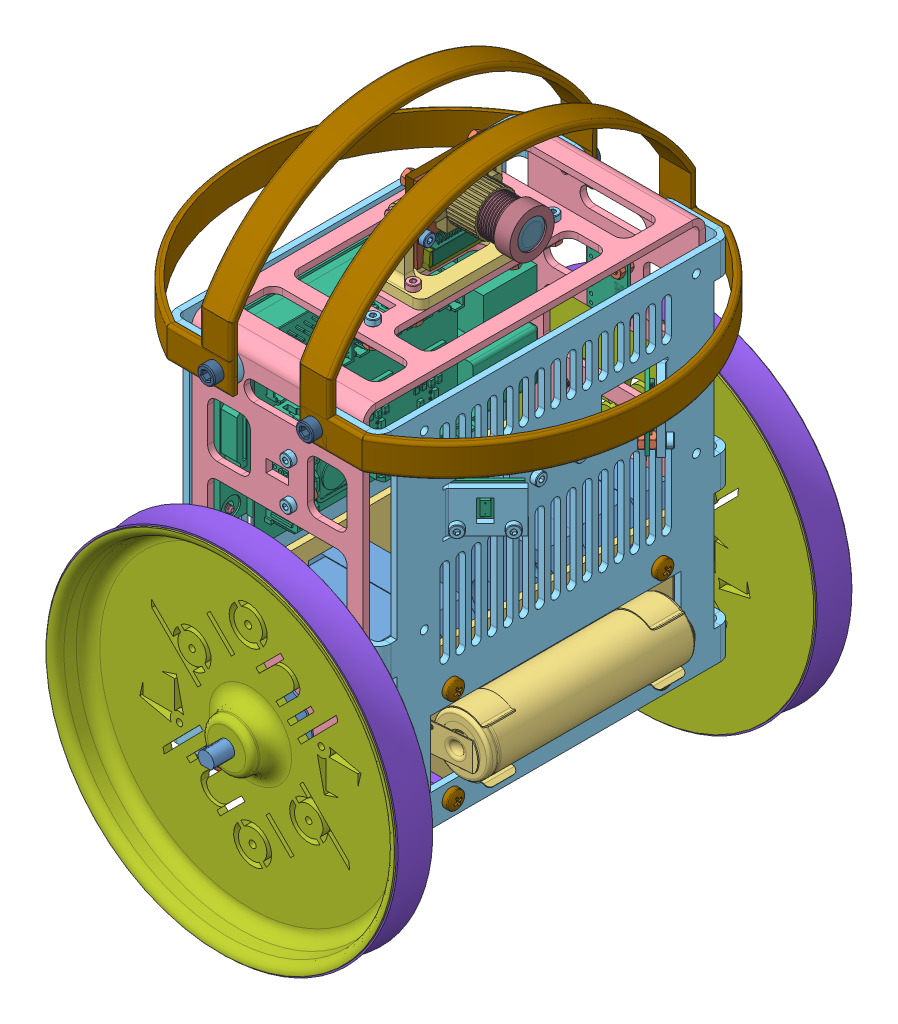
SolidWorks assembly irys4, configuration Domyślna. Lengths in mm.
Overall size (174.89 215.39 153).
175 component instances, 30 part files, 180 mates.
Components (placement in the parent):
- steppermotor-1: steppermotor [Default] at (-42.2578 -7.1789 72.25) size (42.3 42.3 64.5)
- bottomframe_rys3-1: bottomframe_rys3 [Domyślna] at (-43.1924 -30.5373 18.7182) x (0 0 -1) z (0 -1 0) size (108 54 24.86)
- steppermotor-2: steppermotor [Default] at (-42.2578 -7.1789 -31.75) x (-1 0 0) z (0 0 -1) size (42.3 42.3 64.5)
- battery_module-1: battery_module [Domyślna] at (-62.2578 -30.5373 65.25) x (0 0 -1) z (0 -1 0) size (90 40 22.7)
- topframe-1: topframe [Domyślna] at (-42.6117 88.6087 10.8622) x (0 0 -1) z (0 1 0) size (108 54 97.29)
- front-1: front [Domyślna] at (-98.6996 69.3173 29.4239) x (0.707107 0 0.707107) z (0 -1 0) size (94.01 94.01 115)
- rys_PCB_rpi_simple-1: rys_PCB_rpi_simple [Domyślna] at (-55.33 110.1932 110.0692) x (0 -1 0) z (1 0 0) size (61.22 87.74 23.25)
- front-2: front [Domyślna] at (14.1841 69.3173 11.0761) x (-0.707107 0 -0.707107) z (0 -1 0) size (94.01 94.01 115)
- wheel wide wide-1: wheel wide wide [bionik x2] at (-42.2578 18.6 82.75) x (0 0 1) z (-1 0 0) size (12 110 110)
- wheel wide wide-2: wheel wide wide [bionik x2] at (-42.3556 18.5998 -42.5179) x (0 0 -1) z (0.999993 0.003797 0) size (12 110 110)
- tire wide-1: tire wide [Domyślna] at (-42.2578 -7.1789 -35.7326) x (0 0 -1) z (0.906427 0.422363 0) size (11 111 111)
- tire wide-2: tire wide [Domyślna] at (-42.2578 -7.1789 96.4849) x (0 0 -1) z (0.998984 -0.045072 0) size (11 111 111)
- bumper-2: bumper [Domyślna] at (-72.7578 82.3211 20.318) x (0 0 1) z (0 -1 0) size (116 57.13 10)
- bumper-3: bumper [Domyślna] at (-11.7578 82.3211 20.25) x (0 0 1) z (0 1 0) size (116 57.13 10)
- imu-1: imu [Domyślna] at (-53.5985 -9.4799 25.3181) x (-0.019519 0 -0.999809) z (0 -1 0) size (10.16 22.86 2.23)
- camera_mounted-1: camera_mounted [Domyślna] at (-47.1687 108.7904 16.7906) x (0 0 -1) z (0.999935 0.011413 0) size (36.3 30.27 33.11)
  - Camera Module Assem-1: Camera Module Assem [Default] at (-12.4357 -13.5775 -13.0743) size (25 24 24.98)
    - PCB 1-1: PCB 1 [Default] at (8.9736 12.851 19.5114) size (25 24 2.1)
    - Camera Block-1: Camera Block [Default] at (8.9736 15.851 20.5114) size (22 13.5 12.5)
    - Camera end-1: Camera end [Default] at (8.9736 15.851 27.3922) x (0.999924 0.012337 0) z (0 0 1) size (14 14 17.26)
    - Lenz-1: Lenz [Default] at (8.9736 15.851 43.8922) size (9 9 0.5)
    - 15 Pin Ribbon Block Assem-1: 15 Pin Ribbon Block Assem [Default] at (0.7567 20.5462 10.9417) x (1 0 0) z (0 -1 0) size (22 2.5 7)
      - 15 Pin Ribbon Block-1: 15 Pin Ribbon Block [Default] at (8.217 10.8197 14.6952) size (20 2.5 6)
      - Ribbon Clamp-1: Ribbon Clamp [Default] at (8.217 10.8197 14.6952) size (22 2.5 5)
    - 0603 Resistor-1: 0603 Resistor [Default] at (2.3268 23.572 20.4882) size (1.75 0.89 0.66)
    - 0603 Resistor-2: 0603 Resistor [Default] at (4.5768 23.572 20.4882) size (1.75 0.89 0.66)
    - 0603 Resistor-3: 0603 Resistor [Default] at (15.6203 23.5707 20.4857) size (1.75 0.89 0.66)
    - 0603 Resistor-4: 0603 Resistor [Default] at (13.3703 23.5707 20.4857) size (1.75 0.89 0.66)
  - mount-1: mount [Domyślna] at (-15.8432 -12.9016 1.4371) size (25 24 5)
  - M2 x 0.4mm Thread 5mm LONG SOCKET HEAD CAP SCREW-1: M2 x 0.4mm Thread 5mm LONG SOCKET HEAD CAP SCREW [Domyślna] at (7.0379 9.2735 2.5371) x (-0.356462 0.93431 0) z (0 0 -1) size (3.8 3.8 7.09)
  - M2 x 0.4mm Thread 5mm LONG SOCKET HEAD CAP SCREW-2: M2 x 0.4mm Thread 5mm LONG SOCKET HEAD CAP SCREW [Domyślna] at (7.0379 -4.7265 2.5371) x (-0.994039 0.109029 0) z (0 0 -1) size (3.8 3.8 7.09)
  - M2 x 0.4mm Thread 5mm LONG SOCKET HEAD CAP SCREW-3: M2 x 0.4mm Thread 5mm LONG SOCKET HEAD CAP SCREW [Domyślna] at (-13.9621 9.2735 2.5371) x (-0.583934 -0.811801 0) z (0 0 -1) size (3.8 3.8 7.09)
  - M2 x 0.4mm Thread 5mm LONG SOCKET HEAD CAP SCREW-4: M2 x 0.4mm Thread 5mm LONG SOCKET HEAD CAP SCREW [Domyślna] at (-13.9621 -4.7265 2.5371) x (-0.923728 -0.383049 0) z (0 0 -1) size (3.8 3.8 7.09)
  - m2_x_0_4mm_thread_hex_nut-1: m2_x_0_4mm_thread_hex_nut [Domyślna] at (7.0379 9.2735 3.1371) size (4 4.62 1.6)
  - m2_x_0_4mm_thread_hex_nut-2: m2_x_0_4mm_thread_hex_nut [Domyślna] at (7.0379 -4.7265 3.1371) size (4 4.62 1.6)
  - m2_x_0_4mm_thread_hex_nut-3: m2_x_0_4mm_thread_hex_nut [Domyślna] at (-13.9621 -4.7265 3.1371) size (4 4.62 1.6)
  - m2_x_0_4mm_thread_hex_nut-4: m2_x_0_4mm_thread_hex_nut [Domyślna] at (-13.9621 9.2735 3.1371) size (4 4.62 1.6)
  - mount1-1: mount1 [Domyślna] at (7.7442 -6.03 1.3422) x (1 0 0) z (0 -0.011413 0.999935) size (36.3 23 16)
  - M2 x 0.4mm Thread 10mm LONG SOCKET HEAD CAP SCREW-1: M2 x 0.4mm Thread 10mm LONG SOCKET HEAD CAP SCREW [Domyślna] at (1.9591 2.2735 3.9371) x (0 0.966896 -0.255169) z (-1 0 0) size (3.8 3.8 12.09)
  - M2 x 0.4mm Thread 10mm LONG SOCKET HEAD CAP SCREW-2: M2 x 0.4mm Thread 10mm LONG SOCKET HEAD CAP SCREW [Domyślna] at (-8.8833 2.2735 3.9371) x (0 0 -1) z (1 0 0) size (3.8 3.8 12.09)
- bumper-4: bumper [Domyślna] at (-57.7497 97.3211 20.25) x (0 0 1) z (-1 0.000537 0) size (116 57.13 10)
- bumper-5: bumper [Domyślna] at (-26.7108 97.321 20.25) x (0 0 1) z (-0.999995 0.003129 0) size (116 57.13 10)
- m2_x_0_4mm_thread_6mm_long_sock-1: m2_x_0_4mm_thread_6mm_long_sock [Domyślna] at (-11.1317 52.3211 48.7547) x (-0.511229 -0.690862 0.511229) z (-0.707107 0 -0.707107) size (3.8 3.8 8)
- m2_x_0_4mm_thread_6mm_long_sock-2: m2_x_0_4mm_thread_6mm_long_sock [Domyślna] at (-2.1514 52.3211 39.7744) x (-0.511229 -0.690862 0.511229) z (-0.707107 0 -0.707107) size (3.8 3.8 8)
- M2 x 0.4mm Thread 10mm LONG SOCKET HEAD CAP SCREW-1: M2 x 0.4mm Thread 10mm LONG SOCKET HEAD CAP SCREW [Domyślna] at (-66.0454 33.0917 64.6663) x (0 -0.924225 -0.381849) z (1 0 0) size (3.8 3.8 12.09)
- M2 x 0.4mm Thread 10mm LONG SOCKET HEAD CAP SCREW-2: M2 x 0.4mm Thread 10mm LONG SOCKET HEAD CAP SCREW [Domyślna] at (-66.0454 82.1645 64.6663) x (0 -0.924225 -0.381849) z (1 0 0) size (3.8 3.8 12.09)
- ToF_nut-1: ToF_nut [Domyślna] at (-17.0376 55.6897 33.0308) x (0 -1 0) z (0.707107 0 0.707107) size (12.89 18.5 4.22)
  - vl53l1x-1: vl53l1x [Domyślna] at (-6.7913 -9.4823 16.6745) size (12.7 17.78 2.22)
  - m2_x_0_4mm_thread_hex_nut-1: m2_x_0_4mm_thread_hex_nut [Domyślna] at (3.3687 5.7577 15.8745) size (4 4.62 1.6)
  - m2_x_0_4mm_thread_hex_nut-2: m2_x_0_4mm_thread_hex_nut [Domyślna] at (3.3687 -6.9423 15.8745) x (-0.923728 -0.383049 0) z (0 0 -1) size (4 4.62 1.6)
  - m2_x_0_4mm_thread_hex_nut-3: m2_x_0_4mm_thread_hex_nut [Domyślna] at (3.3687 5.7577 18.4945) x (-0.923728 -0.383049 0) z (0 0 -1) size (4 4.62 1.6)
  - m2_x_0_4mm_thread_hex_nut-4: m2_x_0_4mm_thread_hex_nut [Domyślna] at (3.3687 -6.9423 18.4945) x (-0.923728 -0.383049 0) z (0 0 -1) size (4 4.62 1.6)
- ToF_nut-2: ToF_nut [Domyślna] at (-17.6432 55.6897 6.5354) x (0 -1 0) z (0.707107 0 -0.707107) size (12.89 18.5 4.22)
  - vl53l1x-1: vl53l1x [Domyślna] at (-6.7913 -9.4823 16.6745) size (12.7 17.78 2.22)
  - m2_x_0_4mm_thread_hex_nut-1: m2_x_0_4mm_thread_hex_nut [Domyślna] at (3.3687 5.7577 15.8745) size (4 4.62 1.6)
  - m2_x_0_4mm_thread_hex_nut-2: m2_x_0_4mm_thread_hex_nut [Domyślna] at (3.3687 -6.9423 15.8745) x (-0.923728 -0.383049 0) z (0 0 -1) size (4 4.62 1.6)
  - m2_x_0_4mm_thread_hex_nut-3: m2_x_0_4mm_thread_hex_nut [Domyślna] at (3.3687 5.7577 18.4945) x (-0.923728 -0.383049 0) z (0 0 -1) size (4 4.62 1.6)
  - m2_x_0_4mm_thread_hex_nut-4: m2_x_0_4mm_thread_hex_nut [Domyślna] at (3.3687 -6.9423 18.4945) x (-0.923728 -0.383049 0) z (0 0 -1) size (4 4.62 1.6)
- ToF_nut-3: ToF_nut [Domyślna] at (-29.7647 55.6897 19.6577) x (0 -1 0) z (1 0 0) size (12.89 18.5 4.22)
  - vl53l1x-1: vl53l1x [Domyślna] at (-6.7913 -9.4823 16.6745) size (12.7 17.78 2.22)
  - m2_x_0_4mm_thread_hex_nut-1: m2_x_0_4mm_thread_hex_nut [Domyślna] at (3.3687 5.7577 15.8745) size (4 4.62 1.6)
  - m2_x_0_4mm_thread_hex_nut-2: m2_x_0_4mm_thread_hex_nut [Domyślna] at (3.3687 -6.9423 15.8745) x (-0.923728 -0.383049 0) z (0 0 -1) size (4 4.62 1.6)
  - m2_x_0_4mm_thread_hex_nut-3: m2_x_0_4mm_thread_hex_nut [Domyślna] at (3.3687 5.7577 18.4945) x (-0.923728 -0.383049 0) z (0 0 -1) size (4 4.62 1.6)
  - m2_x_0_4mm_thread_hex_nut-4: m2_x_0_4mm_thread_hex_nut [Domyślna] at (3.3687 -6.9423 18.4945) x (-0.923728 -0.383049 0) z (0 0 -1) size (4 4.62 1.6)
- m2_x_0_4mm_thread_6mm_long_sock-3: m2_x_0_4mm_thread_6mm_long_sock [Domyślna] at (-14.4701 52.3211 13.9) x (0 0.924225 0.381849) z (-1 0 0) size (3.8 3.8 8)
- m2_x_0_4mm_thread_6mm_long_sock-4: m2_x_0_4mm_thread_6mm_long_sock [Domyślna] at (-10.8996 52.3211 -8.3508) x (0.65106 0.390182 0.65106) z (-0.707107 0 0.707107) size (3.8 3.8 8)
- m2_x_0_4mm_thread_6mm_long_sock-5: m2_x_0_4mm_thread_6mm_long_sock [Domyślna] at (-14.4701 52.3211 26.6) x (0 0.924225 0.381849) z (-1 0 0) size (3.8 3.8 8)
- m2_x_0_4mm_thread_6mm_long_sock-6: m2_x_0_4mm_thread_6mm_long_sock [Domyślna] at (-1.9194 52.3211 0.6295) x (0.693391 -0.196001 0.693391) z (-0.707107 0 0.707107) size (3.8 3.8 8)
- ToF_nut-4: ToF_nut [Domyślna] at (-41.1264 69.3142 -2.3423) x (1 0 0) z (0 1 0) size (12.89 18.5 4.22)
  - vl53l1x-1: vl53l1x [Domyślna] at (-6.7913 -9.4823 16.6745) size (12.7 17.78 2.22)
  - m2_x_0_4mm_thread_hex_nut-1: m2_x_0_4mm_thread_hex_nut [Domyślna] at (3.3687 5.7577 15.8745) size (4 4.62 1.6)
  - m2_x_0_4mm_thread_hex_nut-2: m2_x_0_4mm_thread_hex_nut [Domyślna] at (3.3687 -6.9423 15.8745) x (-0.923728 -0.383049 0) z (0 0 -1) size (4 4.62 1.6)
  - m2_x_0_4mm_thread_hex_nut-3: m2_x_0_4mm_thread_hex_nut [Domyślna] at (3.3687 5.7577 18.4945) x (-0.923728 -0.383049 0) z (0 0 -1) size (4 4.62 1.6)
  - m2_x_0_4mm_thread_hex_nut-4: m2_x_0_4mm_thread_hex_nut [Domyślna] at (3.3687 -6.9423 18.4945) x (-0.923728 -0.383049 0) z (0 0 -1) size (4 4.62 1.6)
- ToF_nut-5: ToF_nut [Domyślna] at (-41.1264 69.3142 41.6577) x (1 0 0) z (0 1 0) size (12.89 18.5 4.22)
  - vl53l1x-1: vl53l1x [Domyślna] at (-6.7913 -9.4823 16.6745) size (12.7 17.78 2.22)
  - m2_x_0_4mm_thread_hex_nut-1: m2_x_0_4mm_thread_hex_nut [Domyślna] at (3.3687 5.7577 15.8745) size (4 4.62 1.6)
  - m2_x_0_4mm_thread_hex_nut-2: m2_x_0_4mm_thread_hex_nut [Domyślna] at (3.3687 -6.9423 15.8745) x (-0.923728 -0.383049 0) z (0 0 -1) size (4 4.62 1.6)
  - m2_x_0_4mm_thread_hex_nut-3: m2_x_0_4mm_thread_hex_nut [Domyślna] at (3.3687 5.7577 18.4945) x (-0.923728 -0.383049 0) z (0 0 -1) size (4 4.62 1.6)
  - m2_x_0_4mm_thread_hex_nut-4: m2_x_0_4mm_thread_hex_nut [Domyślna] at (3.3687 -6.9423 18.4945) x (-0.923728 -0.383049 0) z (0 0 -1) size (4 4.62 1.6)
- M2 x 0.4mm Thread 10mm LONG SOCKET HEAD CAP SCREW-3: M2 x 0.4mm Thread 10mm LONG SOCKET HEAD CAP SCREW [Domyślna] at (-37.7578 83.6087 4.6) x (0.952226 0 0.305395) z (0 -1 0) size (3.8 3.8 12.09)
- M2 x 0.4mm Thread 10mm LONG SOCKET HEAD CAP SCREW-4: M2 x 0.4mm Thread 10mm LONG SOCKET HEAD CAP SCREW [Domyślna] at (-37.7578 83.6087 35.9) x (0.999568 0 -0.029375) z (0 -1 0) size (3.8 3.8 12.09)
- m2_x_0_4mm_thread_6mm_long_sock-7: m2_x_0_4mm_thread_6mm_long_sock [Domyślna] at (-37.7578 84.6087 48.6) x (-0.868702 0 -0.495335) z (0 -1 0) size (3.8 3.8 8)
- m2_x_0_4mm_thread_6mm_long_sock-8: m2_x_0_4mm_thread_6mm_long_sock [Domyślna] at (-37.7578 84.6087 -8.1) x (-0.837169 0 -0.546944) z (0 -1 0) size (3.8 3.8 8)
- ToF_nut-6: ToF_nut [Domyślna] at (-41.1264 60.9134 52.9555) size (12.89 18.5 4.22)
  - vl53l1x-1: vl53l1x [Domyślna] at (-6.7913 -9.4823 16.6745) size (12.7 17.78 2.22)
  - m2_x_0_4mm_thread_hex_nut-1: m2_x_0_4mm_thread_hex_nut [Domyślna] at (3.3687 5.7577 15.8745) size (4 4.62 1.6)
  - m2_x_0_4mm_thread_hex_nut-2: m2_x_0_4mm_thread_hex_nut [Domyślna] at (3.3687 -6.9423 15.8745) x (-0.923728 -0.383049 0) z (0 0 -1) size (4 4.62 1.6)
  - m2_x_0_4mm_thread_hex_nut-3: m2_x_0_4mm_thread_hex_nut [Domyślna] at (3.3687 5.7577 18.4945) x (-0.923728 -0.383049 0) z (0 0 -1) size (4 4.62 1.6)
  - m2_x_0_4mm_thread_hex_nut-4: m2_x_0_4mm_thread_hex_nut [Domyślna] at (3.3687 -6.9423 18.4945) x (-0.923728 -0.383049 0) z (0 0 -1) size (4 4.62 1.6)
- ToF_nut-7: ToF_nut [Domyślna] at (-41.1264 59.7288 -12.4555) x (1 0 0) z (0 0 -1) size (12.89 18.5 4.22)
  - vl53l1x-1: vl53l1x [Domyślna] at (-6.7913 -9.4823 16.6745) size (12.7 17.78 2.22)
  - m2_x_0_4mm_thread_hex_nut-1: m2_x_0_4mm_thread_hex_nut [Domyślna] at (3.3687 5.7577 15.8745) size (4 4.62 1.6)
  - m2_x_0_4mm_thread_hex_nut-2: m2_x_0_4mm_thread_hex_nut [Domyślna] at (3.3687 -6.9423 15.8745) x (-0.923728 -0.383049 0) z (0 0 -1) size (4 4.62 1.6)
  - m2_x_0_4mm_thread_hex_nut-3: m2_x_0_4mm_thread_hex_nut [Domyślna] at (3.3687 5.7577 18.4945) x (-0.923728 -0.383049 0) z (0 0 -1) size (4 4.62 1.6)
  - m2_x_0_4mm_thread_hex_nut-4: m2_x_0_4mm_thread_hex_nut [Domyślna] at (3.3687 -6.9423 18.4945) x (-0.923728 -0.383049 0) z (0 0 -1) size (4 4.62 1.6)
- ToF_nut-8: ToF_nut [Domyślna] at (-67.478 55.6897 7.4692) x (0 -1 0) z (-0.707107 0 -0.707107) size (12.89 18.5 4.22)
  - vl53l1x-1: vl53l1x [Domyślna] at (-6.7913 -9.4823 16.6745) size (12.7 17.78 2.22)
  - m2_x_0_4mm_thread_hex_nut-1: m2_x_0_4mm_thread_hex_nut [Domyślna] at (3.3687 5.7577 15.8745) size (4 4.62 1.6)
  - m2_x_0_4mm_thread_hex_nut-2: m2_x_0_4mm_thread_hex_nut [Domyślna] at (3.3687 -6.9423 15.8745) x (-0.923728 -0.383049 0) z (0 0 -1) size (4 4.62 1.6)
  - m2_x_0_4mm_thread_hex_nut-3: m2_x_0_4mm_thread_hex_nut [Domyślna] at (3.3687 5.7577 18.4945) x (-0.923728 -0.383049 0) z (0 0 -1) size (4 4.62 1.6)
  - m2_x_0_4mm_thread_hex_nut-4: m2_x_0_4mm_thread_hex_nut [Domyślna] at (3.3687 -6.9423 18.4945) x (-0.923728 -0.383049 0) z (0 0 -1) size (4 4.62 1.6)
- ToF_nut-9: ToF_nut [Domyślna] at (-54.7508 55.6897 20.8423) x (0 -1 0) z (-1 0 0) size (12.89 18.5 4.22)
  - vl53l1x-1: vl53l1x [Domyślna] at (-6.7913 -9.4823 16.6745) size (12.7 17.78 2.22)
  - m2_x_0_4mm_thread_hex_nut-1: m2_x_0_4mm_thread_hex_nut [Domyślna] at (3.3687 5.7577 15.8745) size (4 4.62 1.6)
  - m2_x_0_4mm_thread_hex_nut-2: m2_x_0_4mm_thread_hex_nut [Domyślna] at (3.3687 -6.9423 15.8745) x (-0.923728 -0.383049 0) z (0 0 -1) size (4 4.62 1.6)
  - m2_x_0_4mm_thread_hex_nut-3: m2_x_0_4mm_thread_hex_nut [Domyślna] at (3.3687 5.7577 18.4945) x (-0.923728 -0.383049 0) z (0 0 -1) size (4 4.62 1.6)
  - m2_x_0_4mm_thread_hex_nut-4: m2_x_0_4mm_thread_hex_nut [Domyślna] at (3.3687 -6.9423 18.4945) x (-0.923728 -0.383049 0) z (0 0 -1) size (4 4.62 1.6)
- ToF_nut-10: ToF_nut [Domyślna] at (-66.8723 55.6897 33.9646) x (0 -1 0) z (-0.707107 0 0.707107) size (12.89 18.5 4.22)
  - vl53l1x-1: vl53l1x [Domyślna] at (-6.7913 -9.4823 16.6745) size (12.7 17.78 2.22)
  - m2_x_0_4mm_thread_hex_nut-1: m2_x_0_4mm_thread_hex_nut [Domyślna] at (3.3687 5.7577 15.8745) size (4 4.62 1.6)
  - m2_x_0_4mm_thread_hex_nut-2: m2_x_0_4mm_thread_hex_nut [Domyślna] at (3.3687 -6.9423 15.8745) x (-0.923728 -0.383049 0) z (0 0 -1) size (4 4.62 1.6)
  - m2_x_0_4mm_thread_hex_nut-3: m2_x_0_4mm_thread_hex_nut [Domyślna] at (3.3687 5.7577 18.4945) x (-0.923728 -0.383049 0) z (0 0 -1) size (4 4.62 1.6)
  - m2_x_0_4mm_thread_hex_nut-4: m2_x_0_4mm_thread_hex_nut [Domyślna] at (3.3687 -6.9423 18.4945) x (-0.923728 -0.383049 0) z (0 0 -1) size (4 4.62 1.6)
- m2_x_0_4mm_thread_6mm_long_sock-9: m2_x_0_4mm_thread_6mm_long_sock [Domyślna] at (-73.3839 52.3211 -8.2547) x (0.707107 0 -0.707107) z (0.707107 0 0.707107) size (3.8 3.8 8)
- m2_x_0_4mm_thread_6mm_long_sock-10: m2_x_0_4mm_thread_6mm_long_sock [Domyślna] at (-82.3641 52.3211 0.7256) x (0.403735 0.820972 -0.403735) z (0.707107 0 0.707107) size (3.8 3.8 8)
- m2_x_0_4mm_thread_6mm_long_sock-11: m2_x_0_4mm_thread_6mm_long_sock [Domyślna] at (-70.0454 52.3211 13.9) x (0 -0.924225 -0.381849) z (1 0 0) size (3.8 3.8 8)
- m2_x_0_4mm_thread_6mm_long_sock-12: m2_x_0_4mm_thread_6mm_long_sock [Domyślna] at (-70.0454 52.3211 26.6) x (0 -0.924225 -0.381849) z (1 0 0) size (3.8 3.8 8)
- m2_x_0_4mm_thread_6mm_long_sock-13: m2_x_0_4mm_thread_6mm_long_sock [Domyślna] at (-82.5962 52.3211 39.8705) x (0.184692 -0.965286 0.184692) z (0.707107 0 -0.707107) size (3.8 3.8 8)
- m2_x_0_4mm_thread_6mm_long_sock-14: m2_x_0_4mm_thread_6mm_long_sock [Domyślna] at (-73.6159 52.3211 48.8508) x (-0.648462 -0.398739 -0.648462) z (0.707107 0 -0.707107) size (3.8 3.8 8)
- m2_x_0_4mm_thread_6mm_long_sock-15: m2_x_0_4mm_thread_6mm_long_sock [Domyślna] at (-37.7578 66.6711 68.25) x (-0.262854 -0.964836 0) z (0 0 -1) size (3.8 3.8 8)
- m2_x_0_4mm_thread_6mm_long_sock-16: m2_x_0_4mm_thread_6mm_long_sock [Domyślna] at (-37.7578 53.9711 68.25) x (0.638921 -0.769272 0) z (0 0 -1) size (3.8 3.8 8)
- m2_x_0_4mm_thread_6mm_long_sock-17: m2_x_0_4mm_thread_6mm_long_sock [Domyślna] at (-37.7578 66.6711 -27.75) size (3.8 3.8 8)
- m2_x_0_4mm_thread_6mm_long_sock-18: m2_x_0_4mm_thread_6mm_long_sock [Domyślna] at (-37.7578 53.9711 -27.75) size (3.8 3.8 8)
- H-H_M3x12mm-1: H-H_M3x12mm [Predeterminado] at (-51.2078 -22.4959 17.65) x (0.837169 0 0.546944) z (0.546944 0 -0.837169) size (5.77 12 5)
- H-H_M3x6mm-1: H-H_M3x6mm [Predeterminado] at (-51.2078 -13.4959 17.65) x (0.837169 0 0.546944) z (0.546944 0 -0.837169) size (5.77 6 5)
- pan cross head_am-2: pan cross head_am [B18.6.7M - M3 x 0.5 x 6 Type I Cross Recessed PHMS --6N] at (-51.2078 -7.0799 17.65) x (0 -1 0) z (0 0 1) size (8.37 5.6 5.6)
- battery_module_H-2: battery_module_H [Domyślna] at (13.655 -6.0808 19.8906) x (0 0 1) z (-1 0 0) size (90 40 24.06)
  - battery_module-1: battery_module [Domyślna] at (-44.6406 -21.0981 81.7004) size (90 40 22.7)
  - H-H_M3x6mm-1: H-H_M3x6mm [Predeterminado] at (-32.6406 13.9019 84.7004) x (1 0 0) z (0 1 0) size (5.77 6 5)
  - H-H_M3x6mm-2: H-H_M3x6mm [Predeterminado] at (33.3594 13.9019 84.7004) x (1 0 0) z (0 1 0) size (5.77 6 5)
  - H-H_M3x6mm-3: H-H_M3x6mm [Predeterminado] at (-32.6406 -16.0981 84.7004) x (1 0 0) z (0 -1 0) size (5.77 6 5)
  - H-H_M3x6mm-4: H-H_M3x6mm [Predeterminado] at (33.3594 -16.0981 84.7004) x (1 0 0) z (0 1 0) size (5.77 6 5)
  - pan cross head_am-1: pan cross head_am [B18.6.7M - M3 x 0.5 x 6 Type I Cross Recessed PHMS --6N] at (-32.6406 -16.0981 77.2589) x (0 0 1) z (-1 0 0) size (8.37 5.6 5.6)
  - pan cross head_am-3: pan cross head_am [B18.6.7M - M3 x 0.5 x 6 Type I Cross Recessed PHMS --6N] at (-32.6406 13.9019 77.2589) x (0 0 1) z (-1 0 0) size (8.37 5.6 5.6)
  - pan cross head_am-4: pan cross head_am [B18.6.7M - M3 x 0.5 x 6 Type I Cross Recessed PHMS --6N] at (33.3594 13.9019 77.2589) x (0 0 1) z (-1 0 0) size (8.37 5.6 5.6)
  - pan cross head_am-5: pan cross head_am [B18.6.7M - M3 x 0.5 x 6 Type I Cross Recessed PHMS --6N] at (33.3594 -16.0981 77.2589) x (0 0 1) z (-1 0 0) size (8.37 5.6 5.6)
- pan cross head_am-3: pan cross head_am [B18.6.7M - M3 x 0.5 x 6 Type I Cross Recessed PHMS --6N] at (-78.4454 -22.1789 53.25) size (8.37 5.6 5.6)
- pan cross head_am-4: pan cross head_am [B18.6.7M - M3 x 0.5 x 6 Type I Cross Recessed PHMS --6N] at (-78.4454 7.8211 53.25) size (8.37 5.6 5.6)
- pan cross head_am-5: pan cross head_am [B18.6.7M - M3 x 0.5 x 6 Type I Cross Recessed PHMS --6N] at (-78.4454 7.8211 -12.75) size (8.37 5.6 5.6)
- pan cross head_am-6: pan cross head_am [B18.6.7M - M3 x 0.5 x 6 Type I Cross Recessed PHMS --6N] at (-78.4454 -22.1789 -12.75) size (8.37 5.6 5.6)
- pan cross head_am-7: pan cross head_am [B18.6.7M - M3 x 0.5 x 6 Type I Cross Recessed PHMS --6N] at (-57.2578 -34.9373 53.25) x (0 1 0) z (0 0 1) size (8.37 5.6 5.6)
- pan cross head_am-8: pan cross head_am [B18.6.7M - M3 x 0.5 x 6 Type I Cross Recessed PHMS --6N] at (-27.2578 -34.9373 53.25) x (0 1 0) z (0 0 1) size (8.37 5.6 5.6)
- pan cross head_am-9: pan cross head_am [B18.6.7M - M3 x 0.5 x 6 Type I Cross Recessed PHMS --6N] at (-57.2578 -34.9373 -12.75) x (0 1 0) z (0 0 1) size (8.37 5.6 5.6)
- pan cross head_am-10: pan cross head_am [B18.6.7M - M3 x 0.5 x 6 Type I Cross Recessed PHMS --6N] at (-27.2578 -34.9373 -12.75) x (0 1 0) z (0 0 1) size (8.37 5.6 5.6)
- battery_module_H-3: battery_module_H [Domyślna] at (-98.1705 -8.277 19.8906) x (0 0 1) z (1 0 0) size (90 40 24.06)
  - battery_module-1: battery_module [Domyślna] at (-44.6406 -21.0981 81.7004) size (90 40 22.7)
  - H-H_M3x6mm-1: H-H_M3x6mm [Predeterminado] at (-32.6406 13.9019 84.7004) x (1 0 0) z (0 1 0) size (5.77 6 5)
  - H-H_M3x6mm-2: H-H_M3x6mm [Predeterminado] at (33.3594 13.9019 84.7004) x (1 0 0) z (0 1 0) size (5.77 6 5)
  - H-H_M3x6mm-3: H-H_M3x6mm [Predeterminado] at (-32.6406 -16.0981 84.7004) x (1 0 0) z (0 -1 0) size (5.77 6 5)
  - H-H_M3x6mm-4: H-H_M3x6mm [Predeterminado] at (33.3594 -16.0981 84.7004) x (1 0 0) z (0 1 0) size (5.77 6 5)
  - pan cross head_am-1: pan cross head_am [B18.6.7M - M3 x 0.5 x 6 Type I Cross Recessed PHMS --6N] at (-32.6406 -16.0981 77.2589) x (0 0 1) z (-1 0 0) size (8.37 5.6 5.6)
  - pan cross head_am-3: pan cross head_am [B18.6.7M - M3 x 0.5 x 6 Type I Cross Recessed PHMS --6N] at (-32.6406 13.9019 77.2589) x (0 0 1) z (-1 0 0) size (8.37 5.6 5.6)
  - pan cross head_am-4: pan cross head_am [B18.6.7M - M3 x 0.5 x 6 Type I Cross Recessed PHMS --6N] at (33.3594 13.9019 77.2589) x (0 0 1) z (-1 0 0) size (8.37 5.6 5.6)
  - pan cross head_am-5: pan cross head_am [B18.6.7M - M3 x 0.5 x 6 Type I Cross Recessed PHMS --6N] at (33.3594 -16.0981 77.2589) x (0 0 1) z (-1 0 0) size (8.37 5.6 5.6)
- pan cross head_am-11: pan cross head_am [B18.6.7M - M3 x 0.5 x 6 Type I Cross Recessed PHMS --6N] at (-6.0701 -22.1789 53.25) x (-1 0 0) z (0 0.924225 0.381849) size (8.37 5.6 5.6)
- pan cross head_am-12: pan cross head_am [B18.6.7M - M3 x 0.5 x 6 Type I Cross Recessed PHMS --6N] at (-6.0701 7.8211 53.25) x (-1 0 0) z (0 0.924225 0.381849) size (8.37 5.6 5.6)
- pan cross head_am-13: pan cross head_am [B18.6.7M - M3 x 0.5 x 6 Type I Cross Recessed PHMS --6N] at (-6.0701 7.8211 -12.75) x (-1 0 0) z (0 0.924225 0.381849) size (8.37 5.6 5.6)
- pan cross head_am-14: pan cross head_am [B18.6.7M - M3 x 0.5 x 6 Type I Cross Recessed PHMS --6N] at (-6.0701 -22.1789 -12.75) x (-1 0 0) z (0 0.924225 0.381849) size (8.37 5.6 5.6)
- M3x6-1: M3x6 [Default] at (-57.7578 82.3211 -40.75) x (0 0 1) z (0.923728 0.383049 0) size (9 5.5 5.5)
- M3x6-2: M3x6 [Default] at (-26.7578 82.3211 -40.75) x (0 0 1) z (0.923728 0.383049 0) size (9 5.5 5.5)
- M3x4-1: M3x4 [Default] at (-26.7578 24.3211 -38.75) x (0 0 1) z (0.923728 0.383049 0) size (7 5.5 5.5)
- M3x4-2: M3x4 [Default] at (-57.7578 24.3211 -38.75) x (0 0 1) z (0.923728 0.383049 0) size (7 5.5 5.5)
- M3x8-1: M3x8 [Default] at (-26.7578 8.3211 -36.75) x (0 0 1) z (0.923728 0.383049 0) size (9 5.5 5.5)
- M3x8-2: M3x8 [Default] at (-57.7578 8.3211 -36.75) x (0 0 1) z (0.923728 0.383049 0) size (9 5.5 5.5)
- M3x8-3: M3x8 [Default] at (-26.7578 -22.6789 -38.75) x (0 0 1) z (-0.923728 -0.383049 0) size (9 5.5 5.5)
- M3x8-4: M3x8 [Default] at (-57.7578 -22.6789 -38.75) x (0 0 1) z (0.923728 0.383049 0) size (9 5.5 5.5)
- M3x6-3: M3x6 [Default] at (-57.7578 82.3211 81.318) x (0 0 -1) z (-0.923728 -0.383049 0) size (9 5.5 5.5)
- M3x6-4: M3x6 [Default] at (-26.7578 82.3211 81.25) x (0 0 -1) z (-0.923728 -0.383049 0) size (9 5.5 5.5)
- M3x4-3: M3x4 [Default] at (-57.7578 24.3211 79.25) x (0 0 -1) z (-0.923728 -0.383049 0) size (7 5.5 5.5)
- M3x4-4: M3x4 [Default] at (-26.7578 24.3211 79.25) x (0 0 -1) z (-0.923728 -0.383049 0) size (7 5.5 5.5)
- M3x8-5: M3x8 [Default] at (-57.7578 8.3211 77.25) x (0 0 -1) z (-0.923728 -0.383049 0) size (9 5.5 5.5)
- M3x8-6: M3x8 [Default] at (-26.7578 8.3211 77.25) x (0 0 -1) z (-0.923728 -0.383049 0) size (9 5.5 5.5)
- M3x8-7: M3x8 [Default] at (-57.7578 -22.6789 79.25) x (0 0 -1) z (-0.923728 -0.383049 0) size (9 5.5 5.5)
- M3x8-8: M3x8 [Default] at (-26.7578 -22.6789 79.25) x (0 0 -1) z (-0.923728 -0.383049 0) size (9 5.5 5.5)
Mates (geometry in assembly coordinates):
- Koncentryczne1: concentric aligned: cylinder of steppermotor-1 through (-26.7578 -22.6789 64.75) axis (0 0 1) radius 1.25; cylinder of bottomframe_rys3-1 through (-26.7578 -22.6789 74.25) axis (0 0 1) radius 1.6
- Koncentryczne2: concentric aligned: cylinder of steppermotor-1 through (-57.7578 -22.6789 64.75) axis (0 0 1) radius 1.25; cylinder of bottomframe_rys3-1 through (-57.7578 -22.6789 74.25) axis (0 0 1) radius 1.6
- Wspólnie1: coincident anti-aligned: plane of steppermotor-1 through (-64.2538 -29.1749 72.25) normal (0 0 1); plane of bottomframe_rys3-1 through (-42.2578 -7.6789 72.25) normal (0 0 -1)
- Koncentryczne3: concentric aligned: cylinder of bottomframe_rys3-1 through (-57.7578 -22.6789 -33.75) axis (0 0 -1) radius 1.6; cylinder of steppermotor-2 through (-57.7578 -22.6789 -24.25) axis (0 0 -1) radius 1.25
- Koncentryczne4: concentric aligned: circle of bottomframe_rys3-1; cylinder of steppermotor-2 through (-26.7578 -22.6789 -24.25) axis (0 0 -1) radius 1.25
- Wspólnie2: coincident anti-aligned: plane of bottomframe_rys3-1 through (-42.2578 -159.6789 -31.75) normal (0 0 1); plane of steppermotor-2 through (-20.2618 -29.1749 -31.75) normal (0 0 -1)
- Koncentryczne7: concentric aligned: cylinder of steppermotor-2 through (-26.7578 8.3211 -24.25) axis (0 0 -1) radius 1.25; cylinder of topframe-1 through (-26.7578 8.3211 -33.75) axis (0 0 -1) radius 1.6
- Koncentryczne8: concentric aligned: cylinder of steppermotor-1 through (-57.7578 8.3211 64.75) axis (0 0 1) radius 1.25; cylinder of topframe-1 through (-57.7578 8.3211 74.25) axis (0 0 1) radius 1.6
- Wspólnie4: coincident anti-aligned: plane of steppermotor-1 through (-64.2538 -29.1749 72.25) normal (0 0 1); plane of topframe-1 through (-42.2578 289.3211 72.25) normal (0 0 -1)
- Koncentryczne9: concentric aligned: cylinder of bottomframe_rys3-1 through (-57.7578 -22.6789 74.25) axis (0 0 1) radius 1.6; cylinder of front-1 through (-57.7578 -22.6789 74.25) axis (0 0 1) radius 1.75
- Koncentryczne10: concentric aligned: cylinder of topframe-1 through (-57.7578 82.3211 74.25) axis (0 0 1) radius 1.4; cylinder of front-1 through (-57.7578 82.3211 74.25) axis (0 0 1) radius 1.75
- Koncentryczne11: concentric aligned: cylinder of topframe-1 through (-57.7578 24.3211 -33.75) axis (0 0 -1) radius 1.6; cylinder of front-1 through (-57.7578 24.3211 -33.75) axis (0 0 -1) radius 1.75
- Wspólnie5: coincident anti-aligned: plane of topframe-1 through (-42.2578 -6.6789 -33.75) normal (0 0 -1); plane of front-1 through (-57.7578 82.3211 -33.75) normal (0 0 1)
- Koncentryczne14: concentric aligned: cylinder of front-1 through (-77.0454 82.1645 64.6663) axis (1 0 0) radius 1.25; cylinder of rys_PCB_rpi_simple-1 through (-77.63 82.1645 64.6663) axis (1 0 0) radius 1.375
- Równolegle2: parallel anti-aligned: plane of topframe-1 through (-42.2578 88.6087 -127.75) normal (0 -1 0); plane of rys_PCB_rpi_simple-1 through (-68.63 85.6333 67.9041) normal (0 1 0)
- Koncentryczne17: concentric aligned: cylinder of topframe-1 through (-26.7578 24.3211 -33.75) axis (0 0 -1) radius 1.6; cylinder of front-2 through (-26.7578 24.3211 -33.75) axis (0 0 -1) radius 1.75
- Koncentryczne18: concentric aligned: cylinder of bottomframe_rys3-1 through (-26.7578 -22.6789 -33.75) axis (0 0 -1) radius 1.6; cylinder of steppermotor-2 through (-26.7578 -22.6789 -24.25) axis (0 0 -1) radius 1.25
- Wspólnie8: coincident anti-aligned: plane of topframe-1 through (-42.2578 289.3211 74.25) normal (0 0 1); plane of front-2 through (-26.7578 82.3211 74.25) normal (0 0 -1)
- Koncentryczne19: concentric aligned: cylinder of bottomframe_rys3-1 through (-26.7578 -22.6789 74.25) axis (0 0 1) radius 1.6; cylinder of front-2 through (-26.7578 -22.6789 74.25) axis (0 0 1) radius 1.75
- Koncentryczne26: concentric aligned: cylinder of steppermotor-1 through (-42.2578 -7.1789 72.25) axis (0 0 1) radius 2.5; cylinder of wheel wide wide-1 through (-42.2578 -7.1789 80.25) axis (0 0 1) radius 2.525
- Koncentryczne27: concentric aligned: cylinder of steppermotor-2 through (-42.2578 -7.1789 -31.75) axis (0 0 -1) radius 2.5; cylinder of wheel wide wide-2 through (-42.2578 -7.1789 -40.0179) axis (0 0 -1) radius 2.525
- Koncentryczne29: concentric anti-aligned: cylinder of wheel wide wide-2 through (-42.2578 -7.1789 -50.0179) axis (0 0 -1) radius 53.9972; cylinder of tire wide-1 through (-42.2578 -7.1789 23.9013) axis (0 0 1) radius 53.9972
- Koncentryczne31: concentric aligned: cylinder of wheel wide wide-1 through (-42.2578 -7.1789 90.25) axis (0 0 1) radius 53.9972; circle of tire wide-2
- Koncentryczne36: concentric aligned: cylinder of topframe-1 through (-57.7578 82.3211 74.25) axis (0 0 1) radius 1.4; cylinder of bumper-2 through (-57.7578 82.3211 -37.682) axis (0 0 1) radius 1.5
- Koncentryczne37: concentric aligned: cylinder of topframe-1 through (-26.7578 82.3211 74.25) axis (0 0 1) radius 1.4; cylinder of bumper-3 through (-26.7578 82.3211 -37.75) axis (0 0 1) radius 1.5
- Wspólnie17: coincident anti-aligned: plane of front-2 through (115.2422 82.3211 -35.75) normal (0 0 -1); plane of bumper-3 through (-31.7578 77.3211 -35.75) normal (0 0 1)
- Koncentryczne55: concentric aligned: cylinder of battery_module-1 through (-51.2078 -28.4959 17.65) axis (0 1 0) radius 1.1; cylinder of imu-1 through (-51.2078 -10.4959 17.65) axis (0 1 0) radius 1.0922
- Koncentryczne56: concentric anti-aligned: cylinder of bottomframe_rys3-1 through (-27.2578 -32.5373 53.25) axis (0 -1 0) radius 1.4; cylinder of battery_module-1 through (-27.2578 -28.4959 53.25) axis (0 1 0) radius 1.6
- Koncentryczne57: concentric anti-aligned: cylinder of bottomframe_rys3-1 through (-57.2578 -32.5373 -12.75) axis (0 -1 0) radius 1.4; cylinder of battery_module-1 through (-57.2578 -28.4959 -12.75) axis (0 1 0) radius 1.6
- Wspólnie27: coincident anti-aligned: plane of bottomframe_rys3-1 through (-42.2578 -30.5373 96.25) normal (0 1 0); plane of battery_module-1 through (-62.2578 -30.5373 65.25) normal (0 -1 0)
- Koncentryczne63: concentric aligned: cylinder of topframe-1 through (-37.7578 90.6087 4.6) axis (0 1 0) radius 1.25; cylinder of camera_mounted-1/mount1-1 through (-37.7578 90.6087 4.6) axis (0 1 0) radius 1.05
- Koncentryczne65: concentric aligned: cylinder of topframe-1 through (-37.7578 90.6087 35.9) axis (0 1 0) radius 1.25; cylinder of camera_mounted-1/mount1-1 through (-37.7578 90.6087 35.9) axis (0 1 0) radius 1.05
